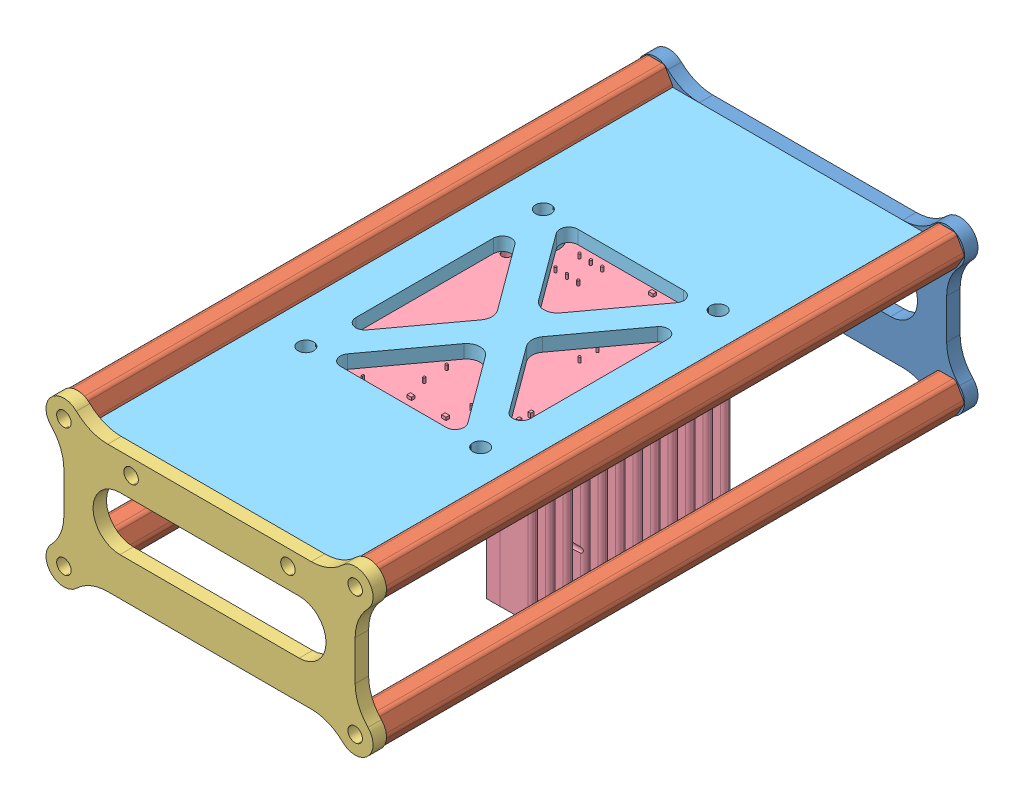
SolidWorks assembly Сборка1, configuration По умолчанию. Lengths in mm.
Overall size (73 36.6 135).
8 component instances, 5 part files, 23 mates.
Components (placement in the parent):
- 65-32.5-3-1: 65-32.5-3 [По умолчанию] at origin size (73 36.5 3)
- stoika-1: stoika [По умолчанию] at (-32.5 0 3) size (7.77 7 129.01)
- stoika-2: stoika [По умолчанию] at (-32.5 28.5 3) size (7.77 7 129.01)
- stoika-3: stoika [По умолчанию] at (32.5 0 3) size (7.77 7 129.01)
- stoika-4: stoika [По умолчанию] at (32.5 28.5 3) size (7.77 7 129.01)
- 65-32.5-3-down-1: 65-32.5-3-down [По умолчанию] at (0 0 132) size (73 36.5 3)
- dc-dc SZBK07-1: dc-dc SZBK07 [По умолчанию] at (0 20.9 67.5) x (-1 0 0) z (0 0 1) size (53.6 27.7 60)
- level-0-2: level-0 [По умолчанию] at (0 25.5 67.5) x (0 0 1) z (0 1 0) size (129 65 7)
Mates (geometry in assembly coordinates):
- Концентричный1: concentric aligned: cylinder of 65-32.5-3-1 through (-32.5 28.5 3) axis (0 0 -1) radius 1.625; cylinder of stoika-2 through (-32.5 28.5 9) axis (0 0 -1) radius 2.25
- Концентричный2: concentric aligned: cylinder of 65-32.5-3-1 through (-32.5 0 3) axis (0 0 -1) radius 1.625; cylinder of stoika-1 through (-32.5 0 9) axis (0 0 -1) radius 2.25
- Концентричный3: concentric aligned: cylinder of 65-32.5-3-1 through (32.5 28.5 3) axis (0 0 -1) radius 1.625; cylinder of stoika-4 through (32.5 28.5 9) axis (0 0 -1) radius 2.25
- Концентричный4: concentric aligned: cylinder of 65-32.5-3-1 through (32.5 0 3) axis (0 0 -1) radius 1.625; cylinder of stoika-3 through (32.5 0 9) axis (0 0 -1) radius 2.25
- Совпадение1: coincident anti-aligned: plane of 65-32.5-3-1 through (0 0 3) normal (0 0 1); plane of stoika-3 through (29.6132 0 3) normal (0 0 -1)
- Совпадение2: coincident anti-aligned: plane of 65-32.5-3-1 through (0 0 3) normal (0 0 1); plane of stoika-4 through (29.6132 28.5 3) normal (0 0 -1)
- Совпадение3: coincident anti-aligned: plane of 65-32.5-3-1 through (0 0 3) normal (0 0 1); plane of stoika-2 through (-35.3868 28.5 3) normal (0 0 -1)
- Совпадение4: coincident anti-aligned: plane of 65-32.5-3-1 through (0 0 3) normal (0 0 1); plane of stoika-1 through (-35.3868 0 3) normal (0 0 -1)
- Параллельность1: parallel aligned: plane of 65-32.5-3-1 through (0 0 3) normal (0 -1 0); plane of stoika-1 through (-33.9434 -3.5 132) normal (0 -1 0)
- Параллельность2: parallel aligned: plane of 65-32.5-3-1 through (0 0 3) normal (0 -1 0); plane of stoika-3 through (31.0566 -3.5 132) normal (0 -1 0)
- Параллельность3: parallel aligned: plane of 65-32.5-3-1 through (0 28.5 3) normal (0 1 0); plane of stoika-4 through (33.9434 32 132) normal (0 1 0)
- Параллельность4: parallel aligned: plane of 65-32.5-3-1 through (0 28.5 3) normal (0 1 0); plane of stoika-2 through (-31.0566 32 132) normal (0 1 0)
- Концентричный5: concentric anti-aligned: cylinder of stoika-3 through (32.5 0 126) axis (0 0 1) radius 2.25; cylinder of 65-32.5-3-down-1 through (32.5 0 135) axis (0 0 -1) radius 1.625
- Концентричный6: concentric anti-aligned: cylinder of stoika-1 through (-32.5 0 126) axis (0 0 1) radius 2.25; cylinder of 65-32.5-3-down-1 through (-32.5 0 135) axis (0 0 -1) radius 1.625
- Совпадение9: coincident anti-aligned: plane of stoika-1 through (-35.3868 0 132) normal (0 0 1); plane of 65-32.5-3-down-1 through (0 0 132) normal (0 0 -1)
- Концентричный7: concentric aligned: cylinder of 65-32.5-3-1 through (17.5 25 10) axis (0 0 -1) radius 1.625; cylinder of level-0-2 through (17.5 25 13) axis (0 0 -1) radius 1.375
- Концентричный8: concentric aligned: cylinder of 65-32.5-3-1 through (-17.5 25 10) axis (0 0 -1) radius 1.625; cylinder of level-0-2 through (-17.5 25 13) axis (0 0 -1) radius 1.375
- Совпадение10: coincident anti-aligned: plane of 65-32.5-3-1 through (0 0 3) normal (0 0 1); plane of level-0-2 through (-32.5 28.5 3) normal (0 0 -1)
- Концентричный9: concentric: cylinder of dc-dc SZBK07-1 through (19.5 12.419 41) axis (0 -1 0) radius 1.6; cylinder of level-0-2 through (19.5 35.5 41) axis (0 -1 0) radius 1.75
- Концентричный10: concentric: cylinder of dc-dc SZBK07-1 through (19.5 12.419 94) axis (0 -1 0) radius 1.6; cylinder of level-0-2 through (19.5 35.5 94) axis (0 -1 0) radius 1.75
- Концентричный11: concentric: cylinder of dc-dc SZBK07-1 through (-19.5 12.419 94) axis (0 -1 0) radius 1.6; cylinder of level-0-2 through (-19.5 35.5 94) axis (0 -1 0) radius 1.75
- Концентричный12: concentric: cylinder of dc-dc SZBK07-1 through (-19.5 12.419 41) axis (0 -1 0) radius 1.6; cylinder of level-0-2 through (-19.5 35.5 41) axis (0 -1 0) radius 1.75
- Совпадение11: coincident anti-aligned: plane of dc-dc SZBK07-1 through (0 22.5 67.5) normal (0 1 0); plane of level-0-2 through (19.5 22.5 41) normal (0 -1 0)
